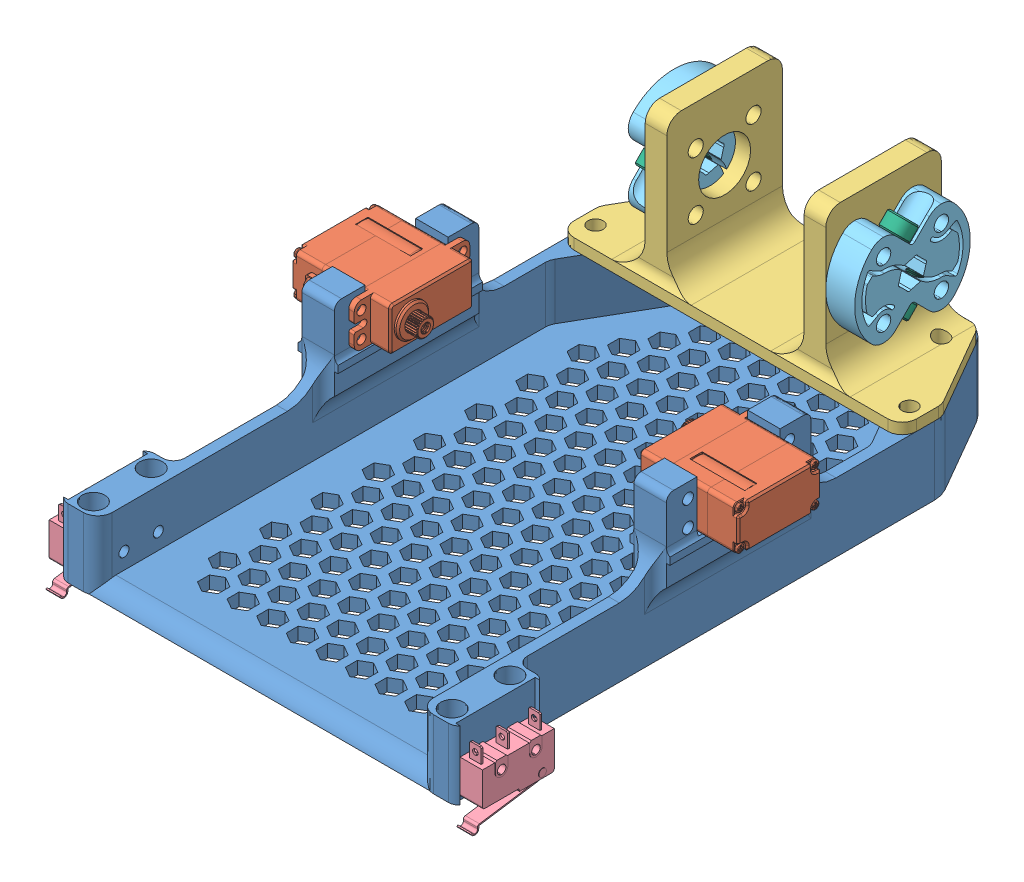
SolidWorks assembly Outtake Bay Assembly, configuration Default. Lengths in mm.
Overall size (123.7 67.29 168.4).
14 component instances, 8 part files, 6 mates.
Components (placement in the parent):
- Outtake Bay Worlds-1: Outtake Bay Worlds [Default] at (57.9469 58.235 69.2067) size (109.78 41.96 168.4)
- Axon_MICRO (1).step-1: Axon_MICRO (1).step [Default] at (15.4969 92.235 139.7535) x (0 0 1) z (0 1 0) size (32 31.6 12)
- Axon_MICRO (1).step-2: Axon_MICRO (1).step [Default] at (100.3969 92.235 139.7535) x (0 0 -1) z (0 1 0) size (32 31.6 12)
- Top Mount for Bay-1: Top Mount for Bay [Default] at (57.9469 77.235 69.2067) size (94.9 43 35.74)
- 3103-0001-0002.step-1: 3103-0001-0002.step [Default] at (1.0754 63.5235 210.241) x (0 0 1) z (0 1 0) size (21.91 6.44 19.81)
- 3103-0001-0002.step-2: 3103-0001-0002.step [Default] at (114.8184 63.5235 210.241) x (0 0 1) z (0 1 0) size (21.91 6.44 19.81)
- rex sonic hub.STEP-1: rex sonic hub.STEP [Default] at (17.7586 82.2088 27.5166) x (0 0 -1) z (1 0 0) size (28.36 32 10.95)
  - 1311-0016-4008.STEP-1: 1311-0016-4008.STEP [Default] at (-46.6459 19.0262 11.1883) size (25.38 32 10)
  - 2800-0004-0014_90128A207.STEP-1: 2800-0004-0014_90128A207.STEP [Default] at (-48.6988 7.9075 11.1883) x (0.5 -0.5 0.707107) z (-0.707107 -0.707107 0) size (7 7 18.01)
  - 2800-0004-0014_90128A207.STEP-2: 2800-0004-0014_90128A207.STEP [Default] at (-44.5931 30.1449 11.1883) x (-0.5 0.5 0.707107) z (0.707107 0.707107 0) size (7 7 18.01)
- rex sonic hub.STEP-2: rex sonic hub.STEP [Default] at (98.1352 147.8809 93.1888) x (0 1 0) z (-1 0 0) size (28.36 32 10.95)
  - 1311-0016-4008.STEP-1: 1311-0016-4008.STEP [Default] at (-46.6459 19.0262 11.1883) size (25.38 32 10)
  - 2800-0004-0014_90128A207.STEP-1: 2800-0004-0014_90128A207.STEP [Default] at (-48.6988 7.9075 11.1883) x (0.5 -0.5 0.707107) z (-0.707107 -0.707107 0) size (7 7 18.01)
  - 2800-0004-0014_90128A207.STEP-2: 2800-0004-0014_90128A207.STEP [Default] at (-44.5931 30.1449 11.1883) x (-0.5 0.5 0.707107) z (0.707107 0.707107 0) size (7 7 18.01)
Mates (geometry in assembly coordinates):
- Concentric1: concentric anti-aligned: cylinder of Top Mount for Bay-1 through (-47.0531 101.235 74.1626) axis (1 0 0) radius 7.2; cylinder of rex sonic hub.STEP-1/1311-0016-4008.STEP-1 through (33.9469 101.235 74.1626) axis (-1 0 0) radius 7
- Concentric2: concentric aligned: cylinder of Top Mount for Bay-1 through (-47.0531 109.235 82.1626) axis (1 0 0) radius 2.1; cylinder of rex sonic hub.STEP-1/1311-0016-4008.STEP-1 through (17.9064 109.235 82.1626) axis (1 0 0) radius 2
- Coincident1: coincident anti-aligned: plane of Top Mount for Bay-1 through (32.9469 120.235 58.1626) normal (-1 0 0); plane of rex sonic hub.STEP-1/1311-0016-4008.STEP-1 through (32.9469 101.235 74.1626) normal (1 0 0)
- Concentric3: concentric aligned: cylinder of Top Mount for Bay-1 through (-47.0531 101.235 74.1626) axis (1 0 0) radius 7.2; cylinder of rex sonic hub.STEP-2/1311-0016-4008.STEP-1 through (81.9469 101.235 74.1626) axis (1 0 0) radius 7
- Concentric4: concentric aligned: circle of Top Mount for Bay-1; cylinder of rex sonic hub.STEP-2/1311-0016-4008.STEP-1 through (97.9874 109.235 66.1626) axis (-1 0 0) radius 2
- Coincident2: coincident anti-aligned: plane of Top Mount for Bay-1 through (82.9469 120.235 58.1626) normal (1 0 0); plane of rex sonic hub.STEP-2/1311-0016-4008.STEP-1 through (82.9469 101.235 74.1626) normal (-1 0 0)
